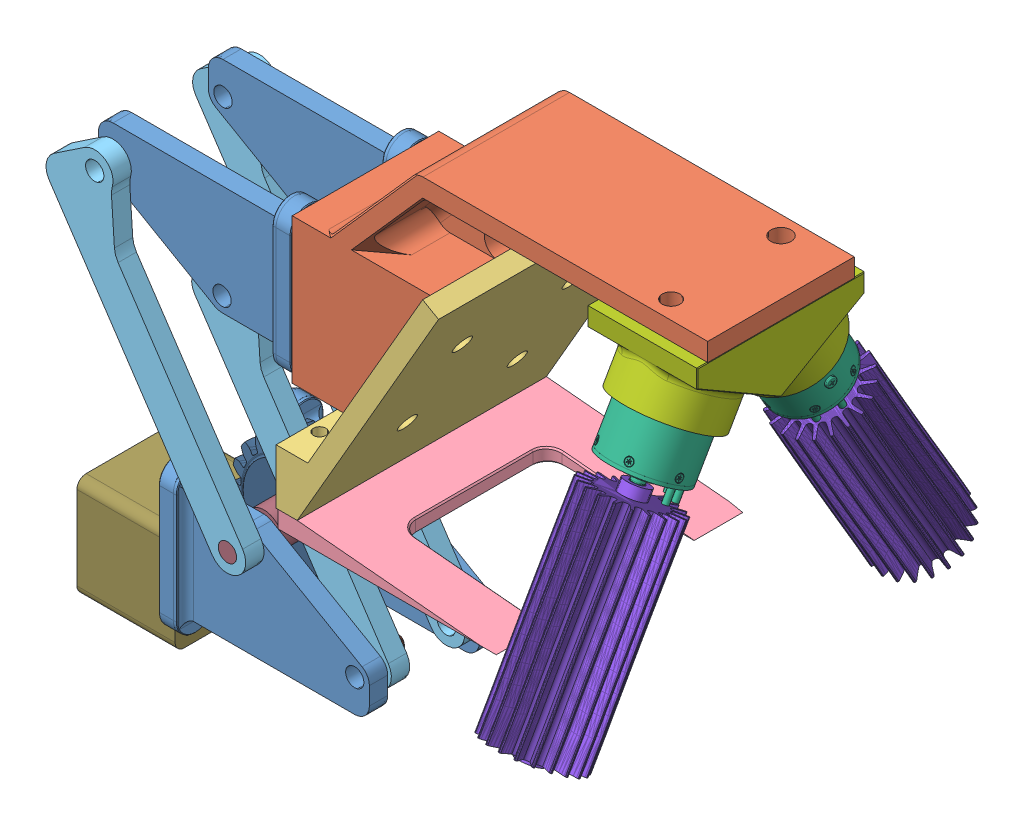
SolidWorks assembly LiftAssy, configuration Default. Lengths in mm.
Overall size (229.52 194.08 170.22).
21 component instances, 13 part files, 41 mates.
Components (placement in the parent):
- LiftLinkageBaseMount-1: LiftLinkageBaseMount [Default] at (120.65 -15.875 60.96) size (69.85 50.85 12.75)
- LiftLinkageBaseMount-2: LiftLinkageBaseMount [Default] at (120.65 -15.875 22.86) size (69.85 50.85 12.75)
- LiftLinkageBaseMount-3: LiftLinkageBaseMount [Default] at (153.714 119.8304 60.96) x (-1 0 0) z (0 0 1) size (69.85 50.85 12.75)
- LiftLinkageBaseMount-4: LiftLinkageBaseMount [Default] at (153.714 119.8304 22.86) x (-1 0 0) z (0 0 1) size (69.85 50.85 12.75)
- PyrIntakeAngledMount-1: PyrIntakeAngledMount [Default] at (185.464 100.7804 70.485) x (-1 0 0) z (0 0 -1) size (144.52 85.09 50.8)
- PyrIntakeBacking-1: PyrIntakeBacking [Default] at (198.164 97.3774 45.085) x (0 0 -1) z (0.866025 -0.5 0) size (86.36 101.6 15.88)
- PyrIntakeForks-1: PyrIntakeForks [Default] at (210.9742 47.0333 45.085) x (0 0 -1) z (0 1 0) size (86.36 75.73 6.35)
- LiftLinkage-6: LiftLinkage [Default] at (141.2859 17.145 22.86) x (-0.830828 -0.556529 0) z (0 0 -1) size (25.4 114.3 6.35)
- LiftLinkage-7: LiftLinkage [Default] at (141.2859 17.145 73.66) x (-0.830828 -0.556529 0) z (0 0 -1) size (25.4 114.3 6.35)
- LiftLinkage-8: LiftLinkage [Default] at (179.07 -4.6697 35.56) x (-0.830828 -0.556529 0) z (0 0 -1) size (25.4 114.3 6.35)
- LiftLinkage-9: LiftLinkage [Default] at (179.07 -4.6697 60.96) x (-0.830828 -0.556529 0) z (0 0 -1) size (25.4 114.3 6.35)
- PyrIntakeFlapperMotor-3: PyrIntakeFlapperMotor [Default] at (285.5319 139.3925 59.596) x (0 -0.866025 0.5) z (0.343501 0.469576 0.81333) size (45.7 26.82 26.82)
- PyrIntakeFlapperMotor-4: PyrIntakeFlapperMotor [Default] at (285.5319 139.3925 30.574) x (0 -0.866025 -0.5) z (-0.923977 -0.191224 0.331209) size (45.7 26.82 26.82)
- PyrIntakeMotorMount-1: PyrIntakeMotorMount [Default] at (304.5819 131.0146 45.085) x (0 0 1) z (-1 0 0) size (70.32 33.98 38.1)
- PyrIntakeRoller-1: PyrIntakeRoller [Default] at (285.5319 78.8205 -4.3972) x (0.918298 -0.197945 0.342851) z (-0.39589 -0.459149 0.795269) size (30.23 75 30.45)
- PyrIntakeRoller-2: PyrIntakeRoller [Default] at (285.5319 78.8205 94.5672) x (0.955222 0.147946 0.256249) z (-0.295891 0.477611 0.827246) size (30.23 75 30.45)
- 57545K527_SPEED-REDUCING WORM GEAR FOR 90 DEG TRANSFER-1: 57545K527_SPEED-REDUCING WORM GEAR FOR 90 DEG TRANSFER [57545K527] at (140.5014 -15.9576 44.6236) x (0 0.051502 -0.998673) z (1 0 0) size (31.13 29.72 30.93)
- 57545K511_SPEED-REDUCING WORM GEAR FOR 90 DEG TRANSFER-cutoff-1: 57545K511_SPEED-REDUCING WORM GEAR FOR 90 DEG TRANSFER-cutoff [57545K511] at (141.2859 17.145 45.4541) x (0.997471 0.071068 0) z (0.071068 -0.997471 0) size (44.78 13.14 44.18)
- RotationBushing-1: RotationBushing [Default] at (113.811 -15.9576 44.6236) x (0 0 -1) z (1 0 0) size (12.7 12.7 53.98)
- 6627T380_POSITION-CONTROL DC MOTOR-1: 6627T380_POSITION-CONTROL DC MOTOR [6627T38] at (111.779 -15.9576 44.6236) x (0 0 -1) z (1 0 0) size (35.31 35.31 49.28)
- PyrIntakeLinkageRod-1: PyrIntakeLinkageRod [Default] at (141.2859 17.145 16.51) size (12.7 12.7 57.15)
Mates (geometry in assembly coordinates):
- Concentric20: concentric aligned: cylinder of LiftLinkageBaseMount-4 through (160.064 81.7304 26.035) axis (-1 0 0) radius 3.175; cylinder of PyrIntakeAngledMount-1 through (172.764 81.7304 26.035) axis (-1 0 0) radius 3.175
- Concentric21: concentric aligned: cylinder of LiftLinkageBaseMount-3 through (160.064 119.8304 64.135) axis (-1 0 0) radius 3.175; cylinder of PyrIntakeAngledMount-1 through (172.764 119.8304 64.135) axis (-1 0 0) radius 3.175
- Coincident23: coincident anti-aligned: plane of LiftLinkageBaseMount-3 through (160.064 119.8304 64.135) normal (1 0 0); plane of PyrIntakeAngledMount-1 through (160.064 75.3804 19.685) normal (-1 0 0)
- Concentric22: concentric anti-aligned: cylinder of PyrIntakeAngledMount-1 through (177.6405 87.2296 64.135) axis (0.866025 -0.5 0) radius 3.175; cylinder of PyrIntakeBacking-1 through (194.1383 77.7046 64.135) axis (-0.866025 0.5 0) radius 3.175
- Concentric23: concentric anti-aligned: cylinder of PyrIntakeAngledMount-1 through (177.6405 87.2296 26.035) axis (0.866025 -0.5 0) radius 3.175; cylinder of PyrIntakeBacking-1 through (194.1383 77.7046 26.035) axis (-0.866025 0.5 0) radius 3.175
- Coincident24: coincident anti-aligned: plane of PyrIntakeAngledMount-1 through (210.864 119.3745 70.485) normal (0.866025 -0.5 0); plane of PyrIntakeBacking-1 through (198.164 97.3774 45.085) normal (-0.866025 0.5 0)
- Concentric24: concentric aligned: cylinder of PyrIntakeBacking-1 through (176.4302 146.134 76.835) axis (0 -1 0) radius 2.1828; cylinder of PyrIntakeForks-1 through (176.4302 53.3833 76.835) axis (0 -1 0) radius 2.1828
- Concentric25: concentric aligned: cylinder of PyrIntakeBacking-1 through (176.4302 146.134 13.335) axis (0 -1 0) radius 2.1828; cylinder of PyrIntakeForks-1 through (176.4302 53.3833 13.335) axis (0 -1 0) radius 2.1828
- Coincident25: coincident anti-aligned: plane of PyrIntakeBacking-1 through (172.764 53.3833 88.265) normal (0 -1 0); plane of PyrIntakeForks-1 through (210.9742 53.3833 45.085) normal (0 1 0)
- Coincident26: coincident anti-aligned: plane of LiftLinkageBaseMount-4 through (153.714 119.8304 22.86) normal (0 0 -1); plane of LiftLinkage-6 through (141.2859 17.145 22.86) normal (0 0 1)
- Concentric26: concentric aligned: cylinder of LiftLinkageBaseMount-4 through (95.294 108.625 19.6607) axis (0 0 1) radius 3.175; cylinder of LiftLinkage-6 through (95.294 108.625 16.51) axis (0 0 1) radius 3.175
- Concentric28: concentric aligned: cylinder of LiftLinkageBaseMount-3 through (133.0781 86.8104 57.7607) axis (0 0 1) radius 3.175; cylinder of LiftLinkageBaseMount-4 through (133.0781 86.8104 19.6607) axis (0 0 1) radius 3.175
- Concentric29: concentric aligned: cylinder of LiftLinkageBaseMount-2 through (141.2859 17.145 19.6607) axis (0 0 1) radius 3.175; cylinder of LiftLinkage-6 through (141.2859 17.145 16.51) axis (0 0 1) radius 3.175
- Concentric30: concentric aligned: cylinder of LiftLinkageBaseMount-3 through (95.294 108.625 57.7607) axis (0 0 1) radius 3.175; cylinder of LiftLinkage-7 through (95.294 108.625 67.31) axis (0 0 1) radius 3.175
- Coincident27: coincident anti-aligned: plane of LiftLinkageBaseMount-3 through (153.714 119.8304 67.31) normal (0 0 1); plane of LiftLinkage-7 through (141.2859 17.145 67.31) normal (0 0 -1)
- Concentric31: concentric aligned: cylinder of LiftLinkageBaseMount-1 through (141.2859 17.145 57.7607) axis (0 0 1) radius 3.175; cylinder of LiftLinkage-7 through (141.2859 17.145 67.31) axis (0 0 1) radius 3.175
- Coincident28: coincident anti-aligned: plane of LiftLinkageBaseMount-1 through (120.65 -15.875 67.31) normal (0 0 1); plane of LiftLinkage-7 through (141.2859 17.145 67.31) normal (0 0 -1)
- Concentric32: concentric aligned: cylinder of LiftLinkageBaseMount-4 through (133.0781 86.8104 19.6607) axis (0 0 1) radius 3.175; cylinder of LiftLinkage-8 through (133.0781 86.8104 29.21) axis (0 0 1) radius 3.175
- Coincident29: coincident anti-aligned: plane of LiftLinkageBaseMount-4 through (153.714 119.8304 29.21) normal (0 0 1); plane of LiftLinkage-8 through (179.07 -4.6697 29.21) normal (0 0 -1)
- Concentric33: concentric aligned: cylinder of LiftLinkageBaseMount-2 through (179.07 -4.6697 19.6607) axis (0 0 1) radius 3.175; cylinder of LiftLinkage-8 through (179.07 -4.6697 29.21) axis (0 0 1) radius 3.175
- Concentric34: concentric aligned: cylinder of LiftLinkageBaseMount-3 through (133.0781 86.8104 57.7607) axis (0 0 1) radius 3.175; cylinder of LiftLinkage-9 through (133.0781 86.8104 54.61) axis (0 0 1) radius 3.175
- Coincident30: coincident anti-aligned: plane of LiftLinkageBaseMount-3 through (153.714 119.8304 60.96) normal (0 0 -1); plane of LiftLinkage-9 through (179.07 -4.6697 60.96) normal (0 0 1)
- Concentric35: concentric aligned: cylinder of LiftLinkageBaseMount-1 through (179.07 -4.6697 57.7607) axis (0 0 1) radius 3.175; cylinder of LiftLinkage-9 through (179.07 -4.6697 54.61) axis (0 0 1) radius 3.175
- Coincident34: coincident anti-aligned: plane of PyrIntakeAngledMount-1 through (185.464 154.1204 19.685) normal (0 -1 0); plane of PyrIntakeMotorMount-1 through (266.4819 154.1204 16.0631) normal (0 1 0)
- Concentric39: concentric aligned: cylinder of PyrIntakeFlapperMotor-3 through (285.5319 137.3091 60.7988) axis (0 0.866025 -0.5) radius 2.0951; cylinder of PyrIntakeRoller-2 through (285.5319 46.3445 113.3172) axis (0 0.866025 -0.5) radius 2.2617
- Coincident35: coincident anti-aligned: circle of PyrIntakeFlapperMotor-3; plane of PyrIntakeRoller-2 through (285.5319 111.2964 75.8172) normal (0 0.866025 -0.5)
- Concentric40: concentric aligned: cylinder of PyrIntakeFlapperMotor-4 through (285.5319 137.3091 29.3712) axis (0 0.866025 0.5) radius 2.0951; cylinder of PyrIntakeRoller-1 through (285.5319 46.3445 -23.1472) axis (0 0.866025 0.5) radius 2.2617
- Coincident36: coincident anti-aligned: circle of PyrIntakeFlapperMotor-4; plane of PyrIntakeRoller-1 through (285.5319 111.2964 14.3528) normal (0 0.866025 0.5)
- Concentric41: concentric aligned: circle of PyrIntakeAngledMount-1; cylinder of PyrIntakeMotorMount-1 through (285.5319 136.3404 64.135) axis (0 1 0) radius 3.175
- Concentric42: concentric aligned: cylinder of PyrIntakeAngledMount-1 through (285.5319 141.4204 26.035) axis (0 1 0) radius 3.5049; cylinder of PyrIntakeMotorMount-1 through (285.5319 136.3404 26.035) axis (0 1 0) radius 3.175
- Concentric43: concentric aligned: cylinder of PyrIntakeFlapperMotor-3 through (285.5319 139.3925 59.596) axis (0 0.866025 -0.5) radius 13.4112; cylinder of PyrIntakeMotorMount-1 through (285.5319 128.3939 65.946) axis (0 0.866025 -0.5) radius 13.97
- Coincident37: coincident anti-aligned: plane of PyrIntakeFlapperMotor-3 through (285.5319 139.3925 59.596) normal (0 0.866025 -0.5); plane of PyrIntakeMotorMount-1 through (266.4819 131.0146 45.085) normal (0 -0.866025 0.5)
- Concentric44: concentric aligned: cylinder of PyrIntakeFlapperMotor-4 through (285.5319 139.3925 30.574) axis (0 0.866025 0.5) radius 13.4112; cylinder of PyrIntakeMotorMount-1 through (285.5319 128.3939 24.224) axis (0 0.866025 0.5) radius 13.97
- Coincident38: coincident anti-aligned: plane of PyrIntakeFlapperMotor-4 through (285.5319 139.3925 30.574) normal (0 0.866025 0.5); plane of PyrIntakeMotorMount-1 through (266.4819 147.7704 16.0631) normal (0 -0.866025 -0.5)
- Concentric46: concentric anti-aligned: cylinder of LiftLinkageBaseMount-2 through (141.2859 17.145 19.6607) axis (0 0 1) radius 3.175; cylinder of 57545K511_SPEED-REDUCING WORM GEAR FOR 90 DEG TRANSFER-cutoff-1 through (141.2859 17.145 -21.9745) axis (0 0 -1) radius 6.35
- Concentric47: concentric anti-aligned: cylinder of 57545K527_SPEED-REDUCING WORM GEAR FOR 90 DEG TRANSFER-1 through (140.5014 -15.9576 44.6236) axis (1 0 0) radius 6.35; cylinder of RotationBushing-1 through (167.786 -15.9576 44.6236) axis (-1 0 0) radius 6.35
- Concentric48: concentric anti-aligned: cylinder of RotationBushing-1 through (167.786 -15.9576 44.6236) axis (-1 0 0) radius 2.54; cylinder of 6627T380_POSITION-CONTROL DC MOTOR-1 through (127.019 -15.9576 44.6236) axis (1 0 0) radius 2.4994
- Coincident40: coincident anti-aligned: plane of RotationBushing-1 through (113.811 -15.9576 44.6236) normal (-1 0 0); plane of 6627T380_POSITION-CONTROL DC MOTOR-1 through (113.811 -15.9576 44.6236) normal (1 0 0)
- Parallel1: parallel anti-aligned: plane of LiftLinkageBaseMount-2 through (114.3 -15.875 26.035) normal (-1 0 0); plane of 6627T380_POSITION-CONTROL DC MOTOR-1 through (111.779 -1.4796 59.1016) normal (1 0 0)
- Concentric49: concentric aligned: cylinder of LiftLinkage-7 through (141.2859 17.145 67.31) axis (0 0 1) radius 3.175; cylinder of PyrIntakeLinkageRod-1 through (141.2859 17.145 60.96) axis (0 0 1) radius 3.175
- Coincident42: coincident aligned: plane of LiftLinkage-7 through (141.2859 17.145 73.66) normal (0 0 1); plane of PyrIntakeLinkageRod-1 through (141.2859 17.145 73.66) normal (0 0 1)
